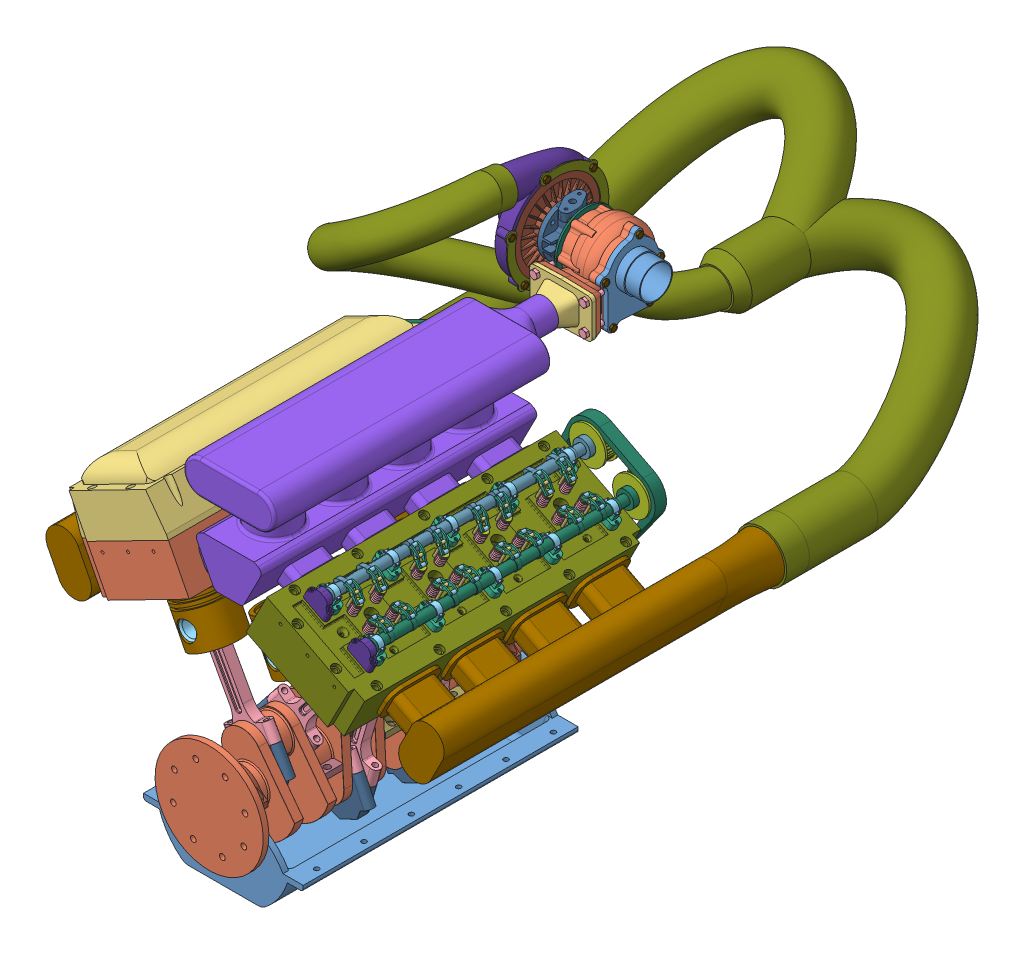
SolidWorks assembly ENSAMBLAJE DE MOTOR V8, configuration Predeterminado. Lengths in mm.
Overall size (718.67 744.91 1254.41).
367 component instances, 54 part files, 489 mates.
Components (placement in the parent):
- BLOQUE V8-1: BLOQUE V8 [Predeterminado] at (-129.263 -163.8973 268.5) size (422.73 344.7 507) (hidden)
- CARTER-1: CARTER [Predeterminado] at (-129.263 -163.8973 268.5) size (280.01 127.77 492.2)
- CIGUEÑAL-1: CIGUEÑAL [Predeterminado] at (-29.5541 -62.6398 687) x (-0.937671 -0.347525 0) z (0 0 1) size (189.6 189.6 554)
- TAPA DE CULATA DERECHO-1: TAPA DE CULATA DERECHO [Predeterminado] at (-262.0137 169.4282 509.5) x (0 0 1) z (-0.890111 -0.455744 0) size (507 100 181.28)
- TAPA DE CULATA IZQUIERDO-1: TAPA DE CULATA IZQUIERDO [Predeterminado] at (233.5589 169.3917 750.5) x (0 0 -1) z (0.890111 -0.455744 0) size (507 100 181.28) (hidden)
- BIELA-4: BIELA [Predeterminado] at (76.4856 71.7664 618.75) x (0.785083 -0.61939 0) z (0 0 1) size (90 198.82 38)
- BULÓN-1: BULÓN [Predeterminado] at (76.4856 71.7664 618.75) x (0.785083 -0.61939 0) z (0 0 1) size (33.8 33.8 75.8)
- COJINETE-1: COJINETE [Predeterminado] at (76.4856 71.7664 618.75) x (0.890111 -0.455744 0) z (0 0 1) size (35.6 35.6 33)
- COJINETE INFERIOR-1: COJINETE INFERIOR [Predeterminado] at (-29.5541 -62.6398 618.75) x (0.890111 -0.455744 0) z (0 0 -1) size (66 33 18)
- COJINETE SUPERIOR-1: COJINETE SUPERIOR [Predeterminado] at (-29.5541 -62.6398 618.75) x (0.890111 -0.455744 0) z (0 0 1) size (66 33 18)
- PISTÓN-1: PISTÓN [Predeterminado] at (62.3575 44.173 618.75) x (0.890111 -0.455744 0) z (0 0 1) size (86 89 88.08)
- SOMBRERETE DE BIELA-1: SOMBRERETE DE BIELA [Predeterminado] at (-29.5541 -62.6398 618.75) x (0.785083 -0.61939 0) z (-0.61939 -0.785083 0) size (90 18.01 61.91)
- BIELA-5: BIELA [Predeterminado] at (75.9097 72.2187 322.75) x (0.787725 -0.616027 0) z (0 0 1) size (90 198.82 38)
- BULÓN-2: BULÓN [Predeterminado] at (75.9097 72.2187 322.75) x (0.787725 -0.616027 0) z (0 0 1) size (33.8 33.8 75.8)
- COJINETE-2: COJINETE [Predeterminado] at (75.9097 72.2187 322.75) x (0.890111 -0.455744 0) z (0 0 1) size (35.6 35.6 33)
- COJINETE INFERIOR-2: COJINETE INFERIOR [Predeterminado] at (-29.5541 -62.6398 322.75) x (0.890111 -0.455744 0) z (0 0 -1) size (66 33 18)
- COJINETE SUPERIOR-2: COJINETE SUPERIOR [Predeterminado] at (-29.5541 -62.6398 322.75) x (0.890111 -0.455744 0) z (0 0 1) size (66 33 18)
- PISTÓN-2: PISTÓN [Predeterminado] at (61.7817 44.6253 322.75) x (0.890111 -0.455744 0) z (0 0 1) size (86 89 88.08)
- SOMBRERETE DE BIELA-2: SOMBRERETE DE BIELA [Predeterminado] at (-29.5541 -62.6398 322.75) x (0.787725 -0.616027 0) z (-0.616027 -0.787725 0) size (90 18.01 61.91)
- BIELA-6: BIELA [Predeterminado] at (-72.3378 9.5283 454.25) x (0.903523 0.428539 0) z (0 0 1) size (90 198.82 38)
- BULÓN-3: BULÓN [Predeterminado] at (-72.3378 9.5283 454.25) x (0.903523 0.428539 0) z (0 0 1) size (33.8 33.8 75.8)
- COJINETE-3: COJINETE [Predeterminado] at (-72.3378 9.5283 454.25) x (0.890111 0.455744 0) z (0 0 1) size (35.6 35.6 33)
- COJINETE INFERIOR-3: COJINETE INFERIOR [Predeterminado] at (1.0281 -145.1549 454.25) x (0.890111 0.455744 0) z (0 0 -1) size (66 33 18)
- COJINETE SUPERIOR-3: COJINETE SUPERIOR [Predeterminado] at (1.0281 -145.1549 454.25) x (0.890111 0.455744 0) z (0 0 1) size (66 33 18)
- PISTÓN-3: PISTÓN [Predeterminado] at (-58.2097 -18.0651 454.25) x (0.890111 0.455744 0) z (0 0 1) size (86 89 88.08)
- SOMBRERETE DE BIELA-3: SOMBRERETE DE BIELA [Predeterminado] at (1.0281 -145.1549 454.25) x (0.903523 0.428539 0) z (0.428539 -0.903523 0) size (90 18.01 61.91)
- BIELA-7: BIELA [Predeterminado] at (71.2823 63.1809 432.75) x (0.970092 -0.242737 0) z (0 0 1) size (90 198.82 38)
- BULÓN-4: BULÓN [Predeterminado] at (71.2823 63.1809 432.75) x (0.970092 -0.242737 0) z (0 0 1) size (33.8 33.8 75.8)
- COJINETE-4: COJINETE [Predeterminado] at (71.2823 63.1809 432.75) x (0.890111 -0.455744 0) z (0 0 1) size (35.6 35.6 33)
- COJINETE INFERIOR-4: COJINETE INFERIOR [Predeterminado] at (29.7257 -102.8988 432.75) x (0.890111 -0.455744 0) z (0 0 -1) size (66 33 18)
- COJINETE SUPERIOR-4: COJINETE SUPERIOR [Predeterminado] at (29.7257 -102.8988 432.75) x (0.890111 -0.455744 0) z (0 0 1) size (66 33 18)
- PISTÓN-4: PISTÓN [Predeterminado] at (57.1543 35.5875 432.75) x (0.890111 -0.455744 0) z (0 0 1) size (86 89 88.08)
- SOMBRERETE DE BIELA-4: SOMBRERETE DE BIELA [Predeterminado] at (29.7257 -102.8988 432.75) x (0.970092 -0.242737 0) z (-0.242737 -0.970092 0) size (90 18.01 61.91)
- BIELA-8: BIELA [Predeterminado] at (-112.163 87.3108 344.25) x (0.87588 0.482529 0) z (0 0 1) size (90 198.82 38)
- BULÓN-5: BULÓN [Predeterminado] at (-112.163 87.3108 344.25) x (0.87588 0.482529 0) z (0 0 1) size (33.8 33.8 75.8)
- COJINETE-5: COJINETE [Predeterminado] at (-112.163 87.3108 344.25) x (0.890111 0.455744 0) z (0 0 1) size (35.6 35.6 33)
- COJINETE INFERIOR-5: COJINETE INFERIOR [Predeterminado] at (-29.5541 -62.6398 344.25) x (0.890111 0.455744 0) z (0 0 -1) size (66 33 18)
- COJINETE SUPERIOR-5: COJINETE SUPERIOR [Predeterminado] at (-29.5541 -62.6398 344.25) x (0.890111 0.455744 0) z (0 0 1) size (66 33 18)
- PISTÓN-5: PISTÓN [Predeterminado] at (-98.035 59.7174 344.25) x (0.890111 0.455744 0) z (0 0 1) size (86 89 88.08)
- SOMBRERETE DE BIELA-5: SOMBRERETE DE BIELA [Predeterminado] at (-29.5541 -62.6398 344.25) x (0.87588 0.482529 0) z (0.482529 -0.87588 0) size (90 18.01 61.91)
- BIELA-9: BIELA [Predeterminado] at (-72.3378 9.5283 564.25) x (0.903523 0.428539 0) z (0 0 1) size (90 198.82 38)
- BULÓN-6: BULÓN [Predeterminado] at (-72.3378 9.5283 564.25) x (0.903523 0.428539 0) z (0 0 1) size (33.8 33.8 75.8)
- COJINETE-6: COJINETE [Predeterminado] at (-72.3378 9.5283 564.25) x (0.890111 0.455744 0) z (0 0 1) size (35.6 35.6 33)
- COJINETE INFERIOR-6: COJINETE INFERIOR [Predeterminado] at (1.0281 -145.1549 564.25) x (0.890111 0.455744 0) z (0 0 -1) size (66 33 18)
- COJINETE SUPERIOR-6: COJINETE SUPERIOR [Predeterminado] at (1.0281 -145.1549 564.25) x (0.890111 0.455744 0) z (0 0 1) size (66 33 18)
- PISTÓN-6: PISTÓN [Predeterminado] at (-58.2097 -18.0651 564.25) x (0.890111 0.455744 0) z (0 0 1) size (86 89 88.08)
- SOMBRERETE DE BIELA-6: SOMBRERETE DE BIELA [Predeterminado] at (1.0281 -145.1549 564.25) x (0.903523 0.428539 0) z (0.428539 -0.903523 0) size (90 18.01 61.91)
- BIELA-10: BIELA [Predeterminado] at (48.7885 19.2483 542.75) x (0.960299 -0.278974 0) z (0 0 1) size (90 198.82 38)
- BULÓN-7: BULÓN [Predeterminado] at (48.7885 19.2483 542.75) x (0.960299 -0.278974 0) z (0 0 1) size (33.8 33.8 75.8)
- COJINETE-7: COJINETE [Predeterminado] at (48.7885 19.2483 542.75) x (0.890111 -0.455744 0) z (0 0 1) size (35.6 35.6 33)
- COJINETE INFERIOR-7: COJINETE INFERIOR [Predeterminado] at (1.0281 -145.1549 542.75) x (0.890111 -0.455744 0) z (0 0 -1) size (66 33 18)
- COJINETE SUPERIOR-7: COJINETE SUPERIOR [Predeterminado] at (1.0281 -145.1549 542.75) x (0.890111 -0.455744 0) z (0 0 1) size (66 33 18)
- PISTÓN-7: PISTÓN [Predeterminado] at (34.6604 -8.3452 542.75) x (0.890111 -0.455744 0) z (0 0 1) size (86 89 88.08)
- SOMBRERETE DE BIELA-7: SOMBRERETE DE BIELA [Predeterminado] at (1.0281 -145.1549 542.75) x (0.960299 -0.278974 0) z (-0.278974 -0.960299 0) size (90 18.01 61.91)
- BIELA-11: BIELA [Predeterminado] at (-112.163 87.3108 676.25) x (0.87588 0.482529 0) z (0 0 1) size (90 198.82 38)
- BULÓN-8: BULÓN [Predeterminado] at (-112.163 87.3108 676.25) x (0.87588 0.482529 0) z (0 0 1) size (33.8 33.8 75.8)
- COJINETE-8: COJINETE [Predeterminado] at (-112.163 87.3108 676.25) x (0.890111 0.455744 0) z (0 0 1) size (35.6 35.6 33)
- COJINETE INFERIOR-8: COJINETE INFERIOR [Predeterminado] at (-29.5541 -62.6398 676.25) x (0.890111 0.455744 0) z (0 0 -1) size (66 33 18)
- COJINETE SUPERIOR-8: COJINETE SUPERIOR [Predeterminado] at (-29.5541 -62.6398 676.25) x (0.890111 0.455744 0) z (0 0 1) size (66 33 18)
- PISTÓN-8: PISTÓN [Predeterminado] at (-98.035 59.7174 676.25) x (0.890111 0.455744 0) z (0 0 1) size (86 89 88.08)
- SOMBRERETE DE BIELA-8: SOMBRERETE DE BIELA [Predeterminado] at (-29.5541 -62.6398 676.25) x (0.87588 0.482529 0) z (0.482529 -0.87588 0) size (90 18.01 61.91)
- SEGURO DE CIGÜEÑAL DE 18mm-1: SEGURO DE CIGÜEÑAL DE 18mm [Predeterminado] at (-14.263 -103.8973 740.5) x (-1 0 0) z (0 0 -1) size (100 42 18)
- SEGURO DE CIGÜEÑAL DE 36mm-1: SEGURO DE CIGÜEÑAL DE 36mm [Predeterminado] at (-14.263 -103.8973 480.5) size (100 42 36)
- SEGURO DE CIGÜEÑAL DE 38mm-1: SEGURO DE CIGÜEÑAL DE 38mm [Predeterminado] at (-14.263 -103.8973 628.5) x (1 0 0) z (0 0 -1) size (100 42 38)
- SEGURO DE CIGÜEÑAL DE 18mm-2: SEGURO DE CIGÜEÑAL DE 18mm [Predeterminado] at (-14.263 -103.8973 296.5) x (-1 0 0) z (0 0 -1) size (100 42 18)
- SEGURO DE CIGÜEÑAL DE 36mm-2: SEGURO DE CIGÜEÑAL DE 36mm [Predeterminado] at (-14.263 -103.8973 406.5) x (1 0 0) z (0 0 -1) size (100 42 36)
- ARBOL DE LEVAS DE ADMISIÓN_IZQUIERDO-2: ARBOL DE LEVAS DE ADMISIÓN_IZQUIERDO [Predeterminado] at (129.8464 248.9794 140.5) x (0 0 -1) z (0.282857 0.959162 0) size (491 30 30)
- ARBOL DE LEVAS DE ESCAPE_IZQUIERDO-2: ARBOL DE LEVAS DE ESCAPE_IZQUIERDO [Predeterminado] at (204.8552 206.8485 140.5) x (0 0 1) z (-0.628385 -0.777902 0) size (491 30 30)
- CULATA_IZQUIERDO-2: CULATA_IZQUIERDO [Predeterminado] at (178.4783 107.717 760.5) x (0 0 -1) z (0.890111 -0.455744 0) size (507 80 181.28)
- SOPORTE EXTERNO DE ARBOL DE LEVAS-1: SOPORTE EXTERNO DE ARBOL DE LEVAS [Predeterminado] at (111.6671 231.8013 707.5) x (0.890111 -0.455744 0) z (0 0 1) size (45 34 11)
- SOPORTE EXTERNO DE ARBOL DE LEVAS-2: SOPORTE EXTERNO DE ARBOL DE LEVAS [Predeterminado] at (188.2167 192.6073 707.5) x (0.890111 -0.455744 0) z (0 0 1) size (45 34 11)
- ARBOL DE LEVAS DE ADMISIÓN_DERECHO-1: ARBOL DE LEVAS DE ADMISIÓN_DERECHO [Predeterminado] at (-142.5063 255.1417 153.25) x (0 0 1) z (0.43783 -0.899058 0) size (511.75 30 30)
- ARBOL DE LEVAS DE ESCAPE_DERECHO-1: ARBOL DE LEVAS DE ESCAPE_DERECHO [Predeterminado] at (-218.2013 211.9839 153.25) x (0 0 -1) z (0.028509 0.999594 0) size (511.75 30 30)
- CULATA_DERECHO-1: CULATA_DERECHO [Predeterminado] at (-64.1949 180.8365 253.5) x (0 0 1) z (-0.890111 -0.455744 0) size (507 80 181.28)
- SOPORTE EXTERNO DE ARBOL DE LEVAS-3: SOPORTE EXTERNO DE ARBOL DE LEVAS [Predeterminado] at (-216.6715 192.6438 728.25) x (0.890111 0.455744 0) z (0 0 1) size (45 34 11)
- SOPORTE EXTERNO DE ARBOL DE LEVAS-4: SOPORTE EXTERNO DE ARBOL DE LEVAS [Predeterminado] at (-140.1219 231.8377 728.25) x (0.890111 0.455744 0) z (0 0 1) size (45 34 11)
- EJE DE CONTROL DE VÁLVULAS-1: EJE DE CONTROL DE VÁLVULAS [Predeterminado] at (-159.7346 199.2777 696.25) x (0 0 -1) z (0.890111 0.455744 0) size (14 48.5 5)
- RESORTE DE VÁLVULA-1: RESORTE DE VÁLVULA [Predeterminado] at (-160.667 210.5262 696.25) x (0 0 -1) z (0.890111 0.455744 0) size (15.13 32.27 14.6)
- SEGUIDOR DE LEVA-1: SEGUIDOR DE LEVA [Predeterminado] at (-166.3151 243.7387 692.45) x (0.994346 0.106192 0) z (0 0 1) size (6 6 7.6)
- SOPORTE DE SEGUIDOR DE VÁLVULA-1: SOPORTE DE SEGUIDOR DE VÁLVULA [Predeterminado] at (-180.6988 240.2228 689.45) x (0.999362 0.035708 0) z (0 0 1) size (30.5 14.83 13.6)
- VÁLVULA-1: VÁLVULA [Predeterminado] at (-129.448 149.5524 696.25) x (0.279369 0.143039 -0.94947) z (0.845134 0.432715 0.313858) size (28 102 28)
- SEGUIDOR DE LEVA-13: SEGUIDOR DE LEVA [Predeterminado] at (-191.9772 233.816 692.45) x (1 0 0) z (0 0 1) size (6 6 7.6)
- EJE DE CONTROL DE VÁLVULAS-2: EJE DE CONTROL DE VÁLVULAS [Predeterminado] at (-149.3077 210.2827 584.25) x (0 0 -1) z (0.890111 0.455744 0) size (14 48.5 5)
- RESORTE DE VÁLVULA-2: RESORTE DE VÁLVULA [Predeterminado] at (-160.3993 210.0033 584.25) x (0 0 -1) z (0.890111 0.455744 0) size (15.13 32.27 14.6)
- SEGUIDOR DE LEVA-17: SEGUIDOR DE LEVA [Predeterminado] at (-158.8913 260.7004 580.45) x (-0.483729 0.875218 0) z (0 0 1) size (6 6 7.6)
- SOPORTE DE SEGUIDOR DE VÁLVULA-2: SOPORTE DE SEGUIDOR DE VÁLVULA [Predeterminado] at (-170.2719 251.2278 577.45) x (0.88227 0.470744 0) z (0 0 1) size (30.5 14.83 13.6)
- VÁLVULA-2: VÁLVULA [Predeterminado] at (-129.1802 149.0296 584.25) x (0.372659 0.190804 -0.908141) z (0.808346 0.413879 0.418665) size (28 102 28)
- SEGUIDOR DE LEVA-21: SEGUIDOR DE LEVA [Predeterminado] at (-177.5936 240.5206 580.45) size (6 6 7.6)
- SEGUIDOR DE LEVA-5: SEGUIDOR DE LEVA [Predeterminado] at (-166.3151 243.7387 652.45) x (0.994346 0.106192 0) z (0 0 1) size (6 6 7.6)
- EJE DE CONTROL DE VÁLVULAS-3: EJE DE CONTROL DE VÁLVULAS [Predeterminado] at (-159.7346 199.2777 656.25) x (0 0 -1) z (0.890111 0.455744 0) size (14 48.5 5)
- SOPORTE DE SEGUIDOR DE VÁLVULA-3: SOPORTE DE SEGUIDOR DE VÁLVULA [Predeterminado] at (-180.6988 240.2228 649.45) x (0.999362 0.035708 0) z (0 0 1) size (30.5 14.83 13.6)
- RESORTE DE VÁLVULA-3: RESORTE DE VÁLVULA [Predeterminado] at (-160.667 210.5262 656.25) x (0 0 -1) z (0.890111 0.455744 0) size (15.13 32.27 14.6)
- VÁLVULA-3: VÁLVULA [Predeterminado] at (-129.448 149.5524 656.25) x (0.279369 0.143039 -0.94947) z (0.845134 0.432715 0.313858) size (28 102 28)
- SEGUIDOR DE LEVA-14: SEGUIDOR DE LEVA [Predeterminado] at (-191.9772 233.816 652.45) x (1 0 0) z (0 0 1) size (6 6 7.6)
- SEGUIDOR DE LEVA-18: SEGUIDOR DE LEVA [Predeterminado] at (-158.8913 260.7004 540.45) x (-0.483729 0.875218 0) z (0 0 1) size (6 6 7.6)
- EJE DE CONTROL DE VÁLVULAS-4: EJE DE CONTROL DE VÁLVULAS [Predeterminado] at (-149.3077 210.2827 544.25) x (0 0 -1) z (0.890111 0.455744 0) size (14 48.5 5)
- SOPORTE DE SEGUIDOR DE VÁLVULA-4: SOPORTE DE SEGUIDOR DE VÁLVULA [Predeterminado] at (-170.2719 251.2278 537.45) x (0.88227 0.470744 0) z (0 0 1) size (30.5 14.83 13.6)
- VÁLVULA-4: VÁLVULA [Predeterminado] at (-129.1802 149.0296 544.25) x (0.372659 0.190804 -0.908141) z (0.808346 0.413879 0.418665) size (28 102 28)
- SEGUIDOR DE LEVA-22: SEGUIDOR DE LEVA [Predeterminado] at (-177.5936 240.5206 540.45) size (6 6 7.6)
- RESORTE DE VÁLVULA-4: RESORTE DE VÁLVULA [Predeterminado] at (-160.3993 210.0033 544.25) x (0 0 -1) z (0.890111 0.455744 0) size (15.13 32.27 14.6)
- SEGUIDOR DE LEVA-12: SEGUIDOR DE LEVA [Predeterminado] at (-166.3151 243.7387 360.45) x (0.994346 0.106192 0) z (0 0 1) size (6 6 7.6)
- EJE DE CONTROL DE VÁLVULAS-5: EJE DE CONTROL DE VÁLVULAS [Predeterminado] at (-159.7346 199.2777 364.25) x (0 0 -1) z (0.890111 0.455744 0) size (14 48.5 5)
- SOPORTE DE SEGUIDOR DE VÁLVULA-5: SOPORTE DE SEGUIDOR DE VÁLVULA [Predeterminado] at (-180.6988 240.2228 357.45) x (0.999362 0.035708 0) z (0 0 1) size (30.5 14.83 13.6)
- RESORTE DE VÁLVULA-5: RESORTE DE VÁLVULA [Predeterminado] at (-160.667 210.5262 364.25) x (0 0 -1) z (0.890111 0.455744 0) size (15.13 32.27 14.6)
- VÁLVULA-5: VÁLVULA [Predeterminado] at (-129.448 149.5524 364.25) x (0.279369 0.143039 -0.94947) z (0.845134 0.432715 0.313858) size (28 102 28)
- SEGUIDOR DE LEVA-16: SEGUIDOR DE LEVA [Predeterminado] at (-191.9772 233.816 360.45) x (1 0 0) z (0 0 1) size (6 6 7.6)
- SEGUIDOR DE LEVA-11: SEGUIDOR DE LEVA [Predeterminado] at (-166.3151 243.7387 320.45) x (0.994346 0.106192 0) z (0 0 1) size (6 6 7.6)
- EJE DE CONTROL DE VÁLVULAS-6: EJE DE CONTROL DE VÁLVULAS [Predeterminado] at (-159.7346 199.2777 324.25) x (0 0 -1) z (0.890111 0.455744 0) size (14 48.5 5)
- SOPORTE DE SEGUIDOR DE VÁLVULA-6: SOPORTE DE SEGUIDOR DE VÁLVULA [Predeterminado] at (-180.6988 240.2228 317.45) x (0.999362 0.035708 0) z (0 0 1) size (30.5 14.83 13.6)
- RESORTE DE VÁLVULA-6: RESORTE DE VÁLVULA [Predeterminado] at (-160.667 210.5262 324.25) x (0 0 -1) z (0.890111 0.455744 0) size (15.13 32.27 14.6)
- VÁLVULA-6: VÁLVULA [Predeterminado] at (-129.448 149.5524 324.25) x (0.279369 0.143039 -0.94947) z (0.845134 0.432715 0.313858) size (28 102 28)
- SEGUIDOR DE LEVA-15: SEGUIDOR DE LEVA [Predeterminado] at (-191.9772 233.816 320.45) x (1 0 0) z (0 0 1) size (6 6 7.6)
- SEGUIDOR DE LEVA-20: SEGUIDOR DE LEVA [Predeterminado] at (-158.8913 260.7004 470.45) x (-0.483729 0.875218 0) z (0 0 1) size (6 6 7.6)
- EJE DE CONTROL DE VÁLVULAS-7: EJE DE CONTROL DE VÁLVULAS [Predeterminado] at (-149.3077 210.2827 474.25) x (0 0 -1) z (0.890111 0.455744 0) size (14 48.5 5)
- SOPORTE DE SEGUIDOR DE VÁLVULA-7: SOPORTE DE SEGUIDOR DE VÁLVULA [Predeterminado] at (-170.2719 251.2278 467.45) x (0.88227 0.470744 0) z (0 0 1) size (30.5 14.83 13.6)
- VÁLVULA-7: VÁLVULA [Predeterminado] at (-129.1802 149.0296 474.25) x (0.372659 0.190804 -0.908141) z (0.808346 0.413879 0.418665) size (28 102 28)
- SEGUIDOR DE LEVA-24: SEGUIDOR DE LEVA [Predeterminado] at (-177.5936 240.5206 470.45) size (6 6 7.6)
- RESORTE DE VÁLVULA-7: RESORTE DE VÁLVULA [Predeterminado] at (-160.3993 210.0033 474.25) x (0 0 -1) z (0.890111 0.455744 0) size (15.13 32.27 14.6)
- SEGUIDOR DE LEVA-19: SEGUIDOR DE LEVA [Predeterminado] at (-158.8913 260.7004 430.45) x (-0.483729 0.875218 0) z (0 0 1) size (6 6 7.6)
- EJE DE CONTROL DE VÁLVULAS-8: EJE DE CONTROL DE VÁLVULAS [Predeterminado] at (-149.3077 210.2827 434.25) x (0 0 -1) z (0.890111 0.455744 0) size (14 48.5 5)
- SOPORTE DE SEGUIDOR DE VÁLVULA-8: SOPORTE DE SEGUIDOR DE VÁLVULA [Predeterminado] at (-170.2719 251.2278 427.45) x (0.88227 0.470744 0) z (0 0 1) size (30.5 14.83 13.6)
- VÁLVULA-8: VÁLVULA [Predeterminado] at (-129.1802 149.0296 434.25) x (0.372659 0.190804 -0.908141) z (0.808346 0.413879 0.418665) size (28 102 28)
- SEGUIDOR DE LEVA-23: SEGUIDOR DE LEVA [Predeterminado] at (-177.5936 240.5206 430.45) size (6 6 7.6)
- RESORTE DE VÁLVULA-8: RESORTE DE VÁLVULA [Predeterminado] at (-160.3993 210.0033 434.25) x (0 0 -1) z (0.890111 0.455744 0) size (15.13 32.27 14.6)
- EJE DE CONTROL DE VÁLVULAS-9: EJE DE CONTROL DE VÁLVULAS [Predeterminado] at (-193.8133 187.4955 696.25) x (0 0 1) z (-0.890111 -0.455744 0) size (14 48.5 5)
- RESORTE DE VÁLVULA-9: RESORTE DE VÁLVULA [Predeterminado] at (-187.3703 196.8538 696.25) x (0.890111 0.455744 0) z (0 0 1) size (15.13 32.27 14.6)
- SEGUIDOR DE LEVA-25: SEGUIDOR DE LEVA [Predeterminado] at (-201.8109 228.7811 700.05) x (0.255826 0.966723 0) z (0 0 -1) size (6 6 7.6)
- SOPORTE DE SEGUIDOR DE VÁLVULA-9: SOPORTE DE SEGUIDOR DE VÁLVULA [Predeterminado] at (-214.7775 228.4406 703.05) x (-0.874136 -0.485681 0) z (0 0 -1) size (30.5 14.83 13.6)
- VÁLVULA-9: VÁLVULA [Predeterminado] at (-156.1513 135.8801 696.25) x (-0.890004 -0.455689 0.015535) z (-0.013828 -0.00708 -0.999879) size (28 102 28)
- SEGUIDOR DE LEVA-34: SEGUIDOR DE LEVA [Predeterminado] at (-228.9095 224.0206 700.05) x (0.999498 -0.031694 0) z (0 0 -1) size (6 6 7.6)
- EJE DE CONTROL DE VÁLVULAS-10: EJE DE CONTROL DE VÁLVULAS [Predeterminado] at (-193.8133 187.4955 584.25) x (0 0 -1) z (0.890111 0.455744 0) size (14 48.5 5)
- RESORTE DE VÁLVULA-10: RESORTE DE VÁLVULA [Predeterminado] at (-187.8751 197.8398 584.25) x (0.873481 0.447229 0.192399) z (-0.171257 -0.087685 0.981317) size (15.13 32.27 14.6)
- SEGUIDOR DE LEVA-38: SEGUIDOR DE LEVA [Predeterminado] at (-228.4393 222.7305 588.05) x (-0.584591 -0.811328 0) z (0 0 -1) size (6 6 7.6)
- SOPORTE DE SEGUIDOR DE VÁLVULA-10: SOPORTE DE SEGUIDOR DE VÁLVULA [Predeterminado] at (-214.7775 228.4406 591.05) x (-0.825387 -0.564567 0) z (0 0 -1) size (30.5 14.83 13.6)
- VÁLVULA-10: VÁLVULA [Predeterminado] at (-156.6561 136.866 584.25) x (0.890111 0.455744 0) z (0 0 1) size (28 102 28)
- SEGUIDOR DE LEVA-42: SEGUIDOR DE LEVA [Predeterminado] at (-201.8981 229.9808 580.45) size (6 6 7.6)
- RESORTE DE VÁLVULA-11: RESORTE DE VÁLVULA [Predeterminado] at (-187.3703 196.8538 656.25) x (0.890111 0.455744 0) z (0 0 1) size (15.13 32.27 14.6) (hidden)
- VÁLVULA-11: VÁLVULA [Predeterminado] at (-156.1513 135.8801 656.25) x (-0.890004 -0.455689 0.015535) z (-0.013828 -0.00708 -0.999879) size (28 102 28) (hidden)
- SEGUIDOR DE LEVA-35: SEGUIDOR DE LEVA [Predeterminado] at (-228.9095 224.0206 660.05) x (0.999498 -0.031694 0) z (0 0 -1) size (6 6 7.6)
- SEGUIDOR DE LEVA-26: SEGUIDOR DE LEVA [Predeterminado] at (-201.8109 228.7811 660.05) x (0.255826 0.966723 0) z (0 0 -1) size (6 6 7.6)
- SOPORTE DE SEGUIDOR DE VÁLVULA-11: SOPORTE DE SEGUIDOR DE VÁLVULA [Predeterminado] at (-214.7775 228.4406 663.05) x (-0.874136 -0.485681 0) z (0 0 -1) size (30.5 14.83 13.6)
- EJE DE CONTROL DE VÁLVULAS-11: EJE DE CONTROL DE VÁLVULAS [Predeterminado] at (-193.8133 187.4955 656.25) x (0 0 1) z (-0.890111 -0.455744 0) size (14 48.5 5)
- VÁLVULA-12: VÁLVULA [Predeterminado] at (-156.6561 136.866 544.25) x (0.890111 0.455744 0) z (0 0 1) size (28 102 28)
- RESORTE DE VÁLVULA-12: RESORTE DE VÁLVULA [Predeterminado] at (-187.8751 197.8398 544.25) x (0.873481 0.447229 0.192399) z (-0.171257 -0.087685 0.981317) size (15.13 32.27 14.6)
- SOPORTE DE SEGUIDOR DE VÁLVULA-12: SOPORTE DE SEGUIDOR DE VÁLVULA [Predeterminado] at (-214.7775 228.4406 551.05) x (-0.825387 -0.564567 0) z (0 0 -1) size (30.5 14.83 13.6)
- SEGUIDOR DE LEVA-39: SEGUIDOR DE LEVA [Predeterminado] at (-228.4393 222.7305 548.05) x (-0.584591 -0.811328 0) z (0 0 -1) size (6 6 7.6)
- EJE DE CONTROL DE VÁLVULAS-12: EJE DE CONTROL DE VÁLVULAS [Predeterminado] at (-193.8133 187.4955 544.25) x (0 0 -1) z (0.890111 0.455744 0) size (14 48.5 5)
- SEGUIDOR DE LEVA-43: SEGUIDOR DE LEVA [Predeterminado] at (-201.8981 229.9808 540.45) size (6 6 7.6)
- VÁLVULA-13: VÁLVULA [Predeterminado] at (-156.6561 136.866 474.25) x (0.890111 0.455744 0) z (0 0 1) size (28 102 28)
- RESORTE DE VÁLVULA-13: RESORTE DE VÁLVULA [Predeterminado] at (-187.8751 197.8398 474.25) x (0.873481 0.447229 0.192399) z (-0.171257 -0.087685 0.981317) size (15.13 32.27 14.6)
- SOPORTE DE SEGUIDOR DE VÁLVULA-13: SOPORTE DE SEGUIDOR DE VÁLVULA [Predeterminado] at (-214.7775 228.4406 481.05) x (-0.825387 -0.564567 0) z (0 0 -1) size (30.5 14.83 13.6)
- SEGUIDOR DE LEVA-41: SEGUIDOR DE LEVA [Predeterminado] at (-228.4393 222.7305 478.05) x (-0.584591 -0.811328 0) z (0 0 -1) size (6 6 7.6)
- EJE DE CONTROL DE VÁLVULAS-13: EJE DE CONTROL DE VÁLVULAS [Predeterminado] at (-193.8133 187.4955 474.25) x (0 0 -1) z (0.890111 0.455744 0) size (14 48.5 5)
- SEGUIDOR DE LEVA-45: SEGUIDOR DE LEVA [Predeterminado] at (-201.8981 229.9808 470.45) size (6 6 7.6)
- VÁLVULA-14: VÁLVULA [Predeterminado] at (-156.6561 136.866 434.25) x (0.890111 0.455744 0) z (0 0 1) size (28 102 28)
- RESORTE DE VÁLVULA-14: RESORTE DE VÁLVULA [Predeterminado] at (-187.8751 197.8398 434.25) x (0.873481 0.447229 0.192399) z (-0.171257 -0.087685 0.981317) size (15.13 32.27 14.6)
- SOPORTE DE SEGUIDOR DE VÁLVULA-14: SOPORTE DE SEGUIDOR DE VÁLVULA [Predeterminado] at (-214.7775 228.4406 441.05) x (-0.825387 -0.564567 0) z (0 0 -1) size (30.5 14.83 13.6)
- SEGUIDOR DE LEVA-40: SEGUIDOR DE LEVA [Predeterminado] at (-228.4393 222.7305 438.05) x (-0.584591 -0.811328 0) z (0 0 -1) size (6 6 7.6)
- EJE DE CONTROL DE VÁLVULAS-14: EJE DE CONTROL DE VÁLVULAS [Predeterminado] at (-193.8133 187.4955 434.25) x (0 0 -1) z (0.890111 0.455744 0) size (14 48.5 5)
- SEGUIDOR DE LEVA-44: SEGUIDOR DE LEVA [Predeterminado] at (-201.8981 229.9808 430.45) size (6 6 7.6)
- RESORTE DE VÁLVULA-15: RESORTE DE VÁLVULA [Predeterminado] at (-187.3703 196.8538 364.25) x (0.890111 0.455744 0) z (0 0 1) size (15.13 32.27 14.6)
- VÁLVULA-15: VÁLVULA [Predeterminado] at (-156.1513 135.8801 364.25) x (-0.890004 -0.455689 0.015535) z (-0.013828 -0.00708 -0.999879) size (28 102 28)
- SEGUIDOR DE LEVA-37: SEGUIDOR DE LEVA [Predeterminado] at (-228.9095 224.0206 368.05) x (0.999498 -0.031694 0) z (0 0 -1) size (6 6 7.6)
- SEGUIDOR DE LEVA-33: SEGUIDOR DE LEVA [Predeterminado] at (-201.8109 228.7811 368.05) x (0.255826 0.966723 0) z (0 0 -1) size (6 6 7.6)
- SOPORTE DE SEGUIDOR DE VÁLVULA-15: SOPORTE DE SEGUIDOR DE VÁLVULA [Predeterminado] at (-214.7775 228.4406 371.05) x (-0.874136 -0.485681 0) z (0 0 -1) size (30.5 14.83 13.6)
- EJE DE CONTROL DE VÁLVULAS-15: EJE DE CONTROL DE VÁLVULAS [Predeterminado] at (-193.8133 187.4955 364.25) x (0 0 1) z (-0.890111 -0.455744 0) size (14 48.5 5)
- RESORTE DE VÁLVULA-16: RESORTE DE VÁLVULA [Predeterminado] at (-187.3703 196.8538 324.25) x (0.890111 0.455744 0) z (0 0 1) size (15.13 32.27 14.6)
- VÁLVULA-16: VÁLVULA [Predeterminado] at (-156.1513 135.8801 324.25) x (-0.890004 -0.455689 0.015535) z (-0.013828 -0.00708 -0.999879) size (28 102 28)
- SEGUIDOR DE LEVA-36: SEGUIDOR DE LEVA [Predeterminado] at (-228.9095 224.0206 328.05) x (0.999498 -0.031694 0) z (0 0 -1) size (6 6 7.6)
- SEGUIDOR DE LEVA-32: SEGUIDOR DE LEVA [Predeterminado] at (-201.8109 228.7811 328.05) x (0.255826 0.966723 0) z (0 0 -1) size (6 6 7.6)
- SOPORTE DE SEGUIDOR DE VÁLVULA-16: SOPORTE DE SEGUIDOR DE VÁLVULA [Predeterminado] at (-214.7775 228.4406 331.05) x (-0.874136 -0.485681 0) z (0 0 -1) size (30.5 14.83 13.6)
- EJE DE CONTROL DE VÁLVULAS-16: EJE DE CONTROL DE VÁLVULAS [Predeterminado] at (-193.8133 187.4955 324.25) x (0 0 1) z (-0.890111 -0.455744 0) size (14 48.5 5)
- EJE DE CONTROL DE VÁLVULAS-17: EJE DE CONTROL DE VÁLVULAS [Predeterminado] at (165.3585 187.459 302.75) x (0 0 -1) z (0.890111 -0.455744 0) size (14 48.5 5)
- RESORTE DE VÁLVULA-17: RESORTE DE VÁLVULA [Predeterminado] at (158.8578 196.7046 302.75) x (0.890111 -0.455744 0) z (0 0 1) size (15.13 32.27 14.6)
- VÁLVULA-18: VÁLVULA [Predeterminado] at (127.6388 135.7308 302.75) x (-0.366338 0.187568 0.911381) z (-0.81123 0.415356 -0.411564) size (28 102 28)
- SEGUIDOR DE LEVA-46: SEGUIDOR DE LEVA [Predeterminado] at (200.5019 224.138 298.95) x (0.783614 -0.621248 0) z (0 0 1) size (6 6 7.6)
- SOPORTE DE SEGUIDOR DE VÁLVULA-19: SOPORTE DE SEGUIDOR DE VÁLVULA [Predeterminado] at (186.3227 228.4041 295.95) x (0.879361 -0.476156 0) z (0 0 1) size (30.5 14.83 13.6)
- SEGUIDOR DE LEVA-53: SEGUIDOR DE LEVA [Predeterminado] at (173.3532 228.6038 298.95) size (6 6 7.6)
- EJE DE CONTROL DE VÁLVULAS-19: EJE DE CONTROL DE VÁLVULAS [Predeterminado] at (165.3585 187.459 412.75) x (0 0 1) z (-0.890111 0.455744 0) size (14 48.5 5)
- RESORTE DE VÁLVULA-19: RESORTE DE VÁLVULA [Predeterminado] at (158.6478 196.2945 412.75) x (0 0 1) z (-0.890111 0.455744 0) size (15.13 32.27 14.6)
- SEGUIDOR DE LEVA-57: SEGUIDOR DE LEVA [Predeterminado] at (200.6612 224.7083 408.95) size (6 6 7.6)
- SOPORTE DE SEGUIDOR DE VÁLVULA-21: SOPORTE DE SEGUIDOR DE VÁLVULA [Predeterminado] at (186.3227 228.4041 405.95) x (0.897697 -0.440613 0) z (0 0 1) size (30.5 14.83 13.6)
- VÁLVULA-20: VÁLVULA [Predeterminado] at (127.4288 135.3208 412.75) x (0.832766 -0.426382 0.353127) z (-0.314323 0.160936 0.935575) size (28 102 28)
- SEGUIDOR DE LEVA-61: SEGUIDOR DE LEVA [Predeterminado] at (173.3555 228.085 408.95) size (6 6 7.6)
- RESORTE DE VÁLVULA-20: RESORTE DE VÁLVULA [Predeterminado] at (158.8578 196.7046 342.75) x (0.890111 -0.455744 0) z (0 0 1) size (15.13 32.27 14.6)
- VÁLVULA-21: VÁLVULA [Predeterminado] at (127.6388 135.7308 342.75) x (-0.366338 0.187568 0.911381) z (-0.81123 0.415356 -0.411564) size (28 102 28)
- SOPORTE DE SEGUIDOR DE VÁLVULA-22: SOPORTE DE SEGUIDOR DE VÁLVULA [Predeterminado] at (186.3227 228.4041 335.95) x (0.879361 -0.476156 0) z (0 0 1) size (30.5 14.83 13.6)
- SEGUIDOR DE LEVA-54: SEGUIDOR DE LEVA [Predeterminado] at (173.3532 228.6038 338.95) size (6 6 7.6)
- EJE DE CONTROL DE VÁLVULAS-20: EJE DE CONTROL DE VÁLVULAS [Predeterminado] at (165.3585 187.459 342.75) x (0 0 -1) z (0.890111 -0.455744 0) size (14 48.5 5)
- SEGUIDOR DE LEVA-47: SEGUIDOR DE LEVA [Predeterminado] at (200.5019 224.138 338.95) x (0.783614 -0.621248 0) z (0 0 1) size (6 6 7.6)
- RESORTE DE VÁLVULA-21: RESORTE DE VÁLVULA [Predeterminado] at (158.6478 196.2945 452.75) x (0 0 1) z (-0.890111 0.455744 0) size (15.13 32.27 14.6)
- VÁLVULA-22: VÁLVULA [Predeterminado] at (127.4288 135.3208 452.75) x (0.832766 -0.426382 0.353127) z (-0.314323 0.160936 0.935575) size (28 102 28)
- SEGUIDOR DE LEVA-62: SEGUIDOR DE LEVA [Predeterminado] at (173.3555 228.085 448.95) size (6 6 7.6)
- SEGUIDOR DE LEVA-58: SEGUIDOR DE LEVA [Predeterminado] at (200.6612 224.7083 448.95) size (6 6 7.6)
- SOPORTE DE SEGUIDOR DE VÁLVULA-23: SOPORTE DE SEGUIDOR DE VÁLVULA [Predeterminado] at (186.3227 228.4041 445.95) x (0.897697 -0.440613 0) z (0 0 1) size (30.5 14.83 13.6)
- EJE DE CONTROL DE VÁLVULAS-21: EJE DE CONTROL DE VÁLVULAS [Predeterminado] at (165.3585 187.459 452.75) x (0 0 1) z (-0.890111 0.455744 0) size (14 48.5 5)
- RESORTE DE VÁLVULA-22: RESORTE DE VÁLVULA [Predeterminado] at (158.6478 196.2945 522.75) x (0 0 1) z (-0.890111 0.455744 0) size (15.13 32.27 14.6)
- VÁLVULA-23: VÁLVULA [Predeterminado] at (127.4288 135.3208 522.75) x (0.832766 -0.426382 0.353127) z (-0.314323 0.160936 0.935575) size (28 102 28)
- SEGUIDOR DE LEVA-64: SEGUIDOR DE LEVA [Predeterminado] at (173.3555 228.085 518.95) size (6 6 7.6)
- SEGUIDOR DE LEVA-60: SEGUIDOR DE LEVA [Predeterminado] at (200.6612 224.7083 518.95) size (6 6 7.6)
- SOPORTE DE SEGUIDOR DE VÁLVULA-24: SOPORTE DE SEGUIDOR DE VÁLVULA [Predeterminado] at (186.3227 228.4041 515.95) x (0.897697 -0.440613 0) z (0 0 1) size (30.5 14.83 13.6)
- EJE DE CONTROL DE VÁLVULAS-22: EJE DE CONTROL DE VÁLVULAS [Predeterminado] at (165.3585 187.459 522.75) x (0 0 1) z (-0.890111 0.455744 0) size (14 48.5 5)
- RESORTE DE VÁLVULA-23: RESORTE DE VÁLVULA [Predeterminado] at (158.6478 196.2945 562.75) x (0 0 1) z (-0.890111 0.455744 0) size (15.13 32.27 14.6)
- VÁLVULA-24: VÁLVULA [Predeterminado] at (127.4288 135.3208 562.75) x (0.832766 -0.426382 0.353127) z (-0.314323 0.160936 0.935575) size (28 102 28)
- SEGUIDOR DE LEVA-63: SEGUIDOR DE LEVA [Predeterminado] at (173.3555 228.085 558.95) size (6 6 7.6)
- SEGUIDOR DE LEVA-59: SEGUIDOR DE LEVA [Predeterminado] at (200.6612 224.7083 558.95) size (6 6 7.6)
- SOPORTE DE SEGUIDOR DE VÁLVULA-25: SOPORTE DE SEGUIDOR DE VÁLVULA [Predeterminado] at (186.3227 228.4041 555.95) x (0.897697 -0.440613 0) z (0 0 1) size (30.5 14.83 13.6)
- EJE DE CONTROL DE VÁLVULAS-23: EJE DE CONTROL DE VÁLVULAS [Predeterminado] at (165.3585 187.459 562.75) x (0 0 1) z (-0.890111 0.455744 0) size (14 48.5 5)
- RESORTE DE VÁLVULA-24: RESORTE DE VÁLVULA [Predeterminado] at (158.8578 196.7046 634.75) x (0.890111 -0.455744 0) z (0 0 1) size (15.13 32.27 14.6)
- VÁLVULA-25: VÁLVULA [Predeterminado] at (127.6388 135.7308 634.75) x (-0.366338 0.187568 0.911381) z (-0.81123 0.415356 -0.411564) size (28 102 28)
- SOPORTE DE SEGUIDOR DE VÁLVULA-26: SOPORTE DE SEGUIDOR DE VÁLVULA [Predeterminado] at (186.3227 228.4041 627.95) x (0.879361 -0.476156 0) z (0 0 1) size (30.5 14.83 13.6)
- SEGUIDOR DE LEVA-56: SEGUIDOR DE LEVA [Predeterminado] at (173.3532 228.6038 630.95) size (6 6 7.6)
- EJE DE CONTROL DE VÁLVULAS-24: EJE DE CONTROL DE VÁLVULAS [Predeterminado] at (165.3585 187.459 634.75) x (0 0 -1) z (0.890111 -0.455744 0) size (14 48.5 5)
- SEGUIDOR DE LEVA-52: SEGUIDOR DE LEVA [Predeterminado] at (200.5019 224.138 630.95) x (0.783614 -0.621248 0) z (0 0 1) size (6 6 7.6)
- RESORTE DE VÁLVULA-25: RESORTE DE VÁLVULA [Predeterminado] at (158.8578 196.7046 674.75) x (0.890111 -0.455744 0) z (0 0 1) size (15.13 32.27 14.6)
- VÁLVULA-26: VÁLVULA [Predeterminado] at (127.6388 135.7308 674.75) x (-0.366338 0.187568 0.911381) z (-0.81123 0.415356 -0.411564) size (28 102 28)
- SOPORTE DE SEGUIDOR DE VÁLVULA-27: SOPORTE DE SEGUIDOR DE VÁLVULA [Predeterminado] at (186.3227 228.4041 667.95) x (0.879361 -0.476156 0) z (0 0 1) size (30.5 14.83 13.6)
- SEGUIDOR DE LEVA-55: SEGUIDOR DE LEVA [Predeterminado] at (173.3532 228.6038 670.95) size (6 6 7.6)
- EJE DE CONTROL DE VÁLVULAS-25: EJE DE CONTROL DE VÁLVULAS [Predeterminado] at (165.3585 187.459 674.75) x (0 0 -1) z (0.890111 -0.455744 0) size (14 48.5 5)
- SEGUIDOR DE LEVA-51: SEGUIDOR DE LEVA [Predeterminado] at (200.5019 224.138 670.95) x (0.783614 -0.621248 0) z (0 0 1) size (6 6 7.6)
- EJE DE CONTROL DE VÁLVULAS-26: EJE DE CONTROL DE VÁLVULAS [Predeterminado] at (120.853 210.2462 674.75) x (0 0 -1) z (0.890111 -0.455744 0) size (14 48.5 5)
- RESORTE DE VÁLVULA-26: RESORTE DE VÁLVULA [Predeterminado] at (132.2122 210.4897 674.75) x (0.361373 -0.185026 -0.913879) z (0.813454 -0.416495 0.405986) size (15.13 32.27 14.6)
- SEGUIDOR DE LEVA-65: SEGUIDOR DE LEVA [Predeterminado] at (129.9696 260.0731 678.55) x (-0.584596 0.811325 0) z (0 0 -1) size (6 6 7.6)
- SOPORTE DE SEGUIDOR DE VÁLVULA-28: SOPORTE DE SEGUIDOR DE VÁLVULA [Predeterminado] at (141.8172 251.1913 681.55) x (-0.905061 0.425281 0) z (0 0 -1) size (30.5 14.83 13.6)
- VÁLVULA-27: VÁLVULA [Predeterminado] at (100.9932 149.516 674.75) x (0.601254 -0.307846 -0.737377) z (0.656347 -0.336055 0.675482) size (28 102 28)
- SEGUIDOR DE LEVA-69: SEGUIDOR DE LEVA [Predeterminado] at (149.6737 240.8702 670.95) size (6 6 7.6)
- EJE DE CONTROL DE VÁLVULAS-27: EJE DE CONTROL DE VÁLVULAS [Predeterminado] at (120.853 210.2462 562.75) x (0 0 -1) z (0.890111 -0.455744 0) size (14 48.5 5)
- RESORTE DE VÁLVULA-27: RESORTE DE VÁLVULA [Predeterminado] at (131.0476 208.2152 562.75) x (0.851719 -0.436086 -0.290524) z (0.258599 -0.132404 0.956868) size (15.13 32.27 14.6)
- SEGUIDOR DE LEVA-73: SEGUIDOR DE LEVA [Predeterminado] at (147.0712 239.3319 566.55) x (0.536876 -0.843661 0) z (0 0 -1) size (6 6 7.6)
- SOPORTE DE SEGUIDOR DE VÁLVULA-29: SOPORTE DE SEGUIDOR DE VÁLVULA [Predeterminado] at (141.8172 251.1913 569.55) x (-0.782036 0.623233 0) z (0 0 -1) size (30.5 14.83 13.6)
- VÁLVULA-28: VÁLVULA [Predeterminado] at (99.8286 147.2414 562.75) x (0.890111 -0.455744 0) z (0 0 1) size (28 102 28)
- SEGUIDOR DE LEVA-77: SEGUIDOR DE LEVA [Predeterminado] at (132.3474 262.5743 558.95) x (1 -0.000048 0) z (0 0 1) size (6 6 7.6)
- VÁLVULA-29: VÁLVULA [Predeterminado] at (100.9932 149.516 634.75) x (0.601254 -0.307846 -0.737377) z (0.656347 -0.336055 0.675482) size (28 102 28)
- RESORTE DE VÁLVULA-28: RESORTE DE VÁLVULA [Predeterminado] at (132.2122 210.4897 634.75) x (0.361373 -0.185026 -0.913879) z (0.813454 -0.416495 0.405986) size (15.13 32.27 14.6)
- SEGUIDOR DE LEVA-66: SEGUIDOR DE LEVA [Predeterminado] at (129.9696 260.0731 638.55) x (-0.584596 0.811325 0) z (0 0 -1) size (6 6 7.6)
- SOPORTE DE SEGUIDOR DE VÁLVULA-30: SOPORTE DE SEGUIDOR DE VÁLVULA [Predeterminado] at (141.8172 251.1913 641.55) x (-0.905061 0.425281 0) z (0 0 -1) size (30.5 14.83 13.6)
- SEGUIDOR DE LEVA-70: SEGUIDOR DE LEVA [Predeterminado] at (149.6737 240.8702 630.95) size (6 6 7.6)
- EJE DE CONTROL DE VÁLVULAS-28: EJE DE CONTROL DE VÁLVULAS [Predeterminado] at (120.853 210.2462 634.75) x (0 0 -1) z (0.890111 -0.455744 0) size (14 48.5 5)
- VÁLVULA-30: VÁLVULA [Predeterminado] at (99.8286 147.2414 522.75) x (0.890111 -0.455744 0) z (0 0 1) size (28 102 28)
- RESORTE DE VÁLVULA-29: RESORTE DE VÁLVULA [Predeterminado] at (131.0476 208.2152 522.75) x (0.851719 -0.436086 -0.290524) z (0.258599 -0.132404 0.956868) size (15.13 32.27 14.6)
- SOPORTE DE SEGUIDOR DE VÁLVULA-31: SOPORTE DE SEGUIDOR DE VÁLVULA [Predeterminado] at (141.8172 251.1913 529.55) x (-0.782036 0.623233 0) z (0 0 -1) size (30.5 14.83 13.6)
- SEGUIDOR DE LEVA-74: SEGUIDOR DE LEVA [Predeterminado] at (147.0712 239.3319 526.55) x (0.536876 -0.843661 0) z (0 0 -1) size (6 6 7.6)
- EJE DE CONTROL DE VÁLVULAS-29: EJE DE CONTROL DE VÁLVULAS [Predeterminado] at (120.853 210.2462 522.75) x (0 0 -1) z (0.890111 -0.455744 0) size (14 48.5 5)
- SEGUIDOR DE LEVA-78: SEGUIDOR DE LEVA [Predeterminado] at (132.3474 262.5743 518.95) x (1 -0.000048 0) z (0 0 1) size (6 6 7.6)
- VÁLVULA-31: VÁLVULA [Predeterminado] at (99.8286 147.2414 452.75) x (0.890111 -0.455744 0) z (0 0 1) size (28 102 28)
- RESORTE DE VÁLVULA-30: RESORTE DE VÁLVULA [Predeterminado] at (131.0476 208.2152 452.75) x (0.851719 -0.436086 -0.290524) z (0.258599 -0.132404 0.956868) size (15.13 32.27 14.6)
- SOPORTE DE SEGUIDOR DE VÁLVULA-32: SOPORTE DE SEGUIDOR DE VÁLVULA [Predeterminado] at (141.8172 251.1913 459.55) x (-0.782036 0.623233 0) z (0 0 -1) size (30.5 14.83 13.6)
- SEGUIDOR DE LEVA-76: SEGUIDOR DE LEVA [Predeterminado] at (147.0712 239.3319 456.55) x (0.536876 -0.843661 0) z (0 0 -1) size (6 6 7.6)
- EJE DE CONTROL DE VÁLVULAS-30: EJE DE CONTROL DE VÁLVULAS [Predeterminado] at (120.853 210.2462 452.75) x (0 0 -1) z (0.890111 -0.455744 0) size (14 48.5 5)
- SEGUIDOR DE LEVA-80: SEGUIDOR DE LEVA [Predeterminado] at (132.3474 262.5743 448.95) x (1 -0.000048 0) z (0 0 1) size (6 6 7.6)
- VÁLVULA-32: VÁLVULA [Predeterminado] at (99.8286 147.2414 412.75) x (0.890111 -0.455744 0) z (0 0 1) size (28 102 28)
- RESORTE DE VÁLVULA-31: RESORTE DE VÁLVULA [Predeterminado] at (131.0476 208.2152 412.75) x (0.851719 -0.436086 -0.290524) z (0.258599 -0.132404 0.956868) size (15.13 32.27 14.6)
- SOPORTE DE SEGUIDOR DE VÁLVULA-33: SOPORTE DE SEGUIDOR DE VÁLVULA [Predeterminado] at (141.8172 251.1913 419.55) x (-0.782036 0.623233 0) z (0 0 -1) size (30.5 14.83 13.6)
- SEGUIDOR DE LEVA-75: SEGUIDOR DE LEVA [Predeterminado] at (147.0712 239.3319 416.55) x (0.536876 -0.843661 0) z (0 0 -1) size (6 6 7.6)
- EJE DE CONTROL DE VÁLVULAS-31: EJE DE CONTROL DE VÁLVULAS [Predeterminado] at (120.853 210.2462 412.75) x (0 0 -1) z (0.890111 -0.455744 0) size (14 48.5 5)
- SEGUIDOR DE LEVA-79: SEGUIDOR DE LEVA [Predeterminado] at (132.3474 262.5743 408.95) x (1 -0.000048 0) z (0 0 1) size (6 6 7.6)
- VÁLVULA-33: VÁLVULA [Predeterminado] at (100.9932 149.516 342.75) x (0.601254 -0.307846 -0.737377) z (0.656347 -0.336055 0.675482) size (28 102 28)
- RESORTE DE VÁLVULA-32: RESORTE DE VÁLVULA [Predeterminado] at (132.2122 210.4897 342.75) x (0.361373 -0.185026 -0.913879) z (0.813454 -0.416495 0.405986) size (15.13 32.27 14.6)
- SEGUIDOR DE LEVA-68: SEGUIDOR DE LEVA [Predeterminado] at (129.9696 260.0731 346.55) x (-0.584596 0.811325 0) z (0 0 -1) size (6 6 7.6)
- SOPORTE DE SEGUIDOR DE VÁLVULA-34: SOPORTE DE SEGUIDOR DE VÁLVULA [Predeterminado] at (141.8172 251.1913 349.55) x (-0.905061 0.425281 0) z (0 0 -1) size (30.5 14.83 13.6)
- SEGUIDOR DE LEVA-72: SEGUIDOR DE LEVA [Predeterminado] at (149.6737 240.8702 338.95) size (6 6 7.6)
- EJE DE CONTROL DE VÁLVULAS-32: EJE DE CONTROL DE VÁLVULAS [Predeterminado] at (120.853 210.2462 342.75) x (0 0 -1) z (0.890111 -0.455744 0) size (14 48.5 5)
- VÁLVULA-34: VÁLVULA [Predeterminado] at (100.9932 149.516 302.75) x (0.601254 -0.307846 -0.737377) z (0.656347 -0.336055 0.675482) size (28 102 28)
- RESORTE DE VÁLVULA-33: RESORTE DE VÁLVULA [Predeterminado] at (132.2122 210.4897 302.75) x (0.361373 -0.185026 -0.913879) z (0.813454 -0.416495 0.405986) size (15.13 32.27 14.6)
- SEGUIDOR DE LEVA-67: SEGUIDOR DE LEVA [Predeterminado] at (129.9696 260.0731 306.55) x (-0.584596 0.811325 0) z (0 0 -1) size (6 6 7.6)
- SOPORTE DE SEGUIDOR DE VÁLVULA-35: SOPORTE DE SEGUIDOR DE VÁLVULA [Predeterminado] at (141.8172 251.1913 309.55) x (-0.905061 0.425281 0) z (0 0 -1) size (30.5 14.83 13.6)
- SEGUIDOR DE LEVA-71: SEGUIDOR DE LEVA [Predeterminado] at (149.6737 240.8702 298.95) size (6 6 7.6)
- EJE DE CONTROL DE VÁLVULAS-33: EJE DE CONTROL DE VÁLVULAS [Predeterminado] at (120.853 210.2462 302.75) x (0 0 -1) z (0.890111 -0.455744 0) size (14 48.5 5)
- MULTIPLE DE ADMISIÓN-1: MULTIPLE DE ADMISIÓN [Predeterminado] at (-77.9978 24.4853 27.5) x (0 0 1) z (-0.890111 0.455744 0) size (553.5 227.32 198.21)
- MULTIPLE DE ESCAPE-1: MULTIPLE DE ESCAPE [Predeterminado] at (-167.0993 -125.6596 27.5) x (0 0 1) z (-0.890111 -0.455744 0) size (626 104.06 121.72)
- MULTIPLE DE ESCAPE-2: MULTIPLE DE ESCAPE [Predeterminado] at (376.4675 338.7952 6) x (0 0 1) z (0.890111 -0.455744 0) size (626 104.06 121.72)
- ENSAMBLAJE TURBO-1: ENSAMBLAJE TURBO [Predeterminado] at (-140.4956 322.1174 236.0327) x (0 0.000002 1) z (-0.999999 -0.001049 0) size (255.82 249.71 242.14)
  - CUBIERTA-1: CUBIERTA [Predeterminado] at (-161.1371 63.4758 -92.0191) size (86.36 103.34 67.62)
  - PLATO DEL COMPRESOR-1: PLATO DEL COMPRESOR [Predeterminado] at (-161.1371 63.4758 -35.6311) x (-0.919239 -0.393701 0) z (0 0 1) size (155.96 155.96 21.59)
  - CARRERA DE EMPUJE-3: CARRERA DE EMPUJE [Predeterminado] at (-161.1371 63.4758 -34.3611) size (24.13 24.13 16.51)
  - TURBINA-1: TURBINA [Predeterminado] at (-161.1371 63.4758 -27.5031) x (0.213829 -0.976871 0) z (0 0 1) size (74.17 77.91 38.1)
  - RUEDA DE TURBINA-1: RUEDA DE TURBINA [Predeterminado] at (-161.1371 63.4758 -148.9151) x (0.213829 -0.976871 0) z (0 0 1) size (59.59 60.38 174.75)
  - ABRAZADERA DE CUBIERTA DE TURBINA-1: ABRAZADERA DE CUBIERTA DE TURBINA [Predeterminado] at (-161.1371 63.4758 -88.2091) x (-1 0.000002 0) z (0 0 1) size (106.65 53.34 3.3)
  - ABRAZADERA DE CUBIERTA DE TURBINA-2: ABRAZADERA DE CUBIERTA DE TURBINA [Predeterminado] at (-161.1371 63.4758 -84.9071) x (-1 0.000353 0) z (0 0 -1) size (106.65 53.34 3.3)
  - PINZA DE COMPRESOR-1: PINZA DE COMPRESOR [Predeterminado] at (-161.1371 63.4758 -37.5361) x (0.702176 0.712004 0) z (0 0 1) size (165.34 61.29 1.91)
  - SELLO DEL COMPRESOR-1: SELLO DEL COMPRESOR [Predeterminado] at (-161.1371 63.476 -11.5011) x (0.991033 0.133614 0) z (0 0 1) size (202.53 187.91 71.74)
  - PINZA DE COMPRESOR-2: PINZA DE COMPRESOR [Predeterminado] at (-161.1372 63.4758 -37.5361) x (-0.702174 -0.712005 0) z (0 0 1) size (165.34 61.29 1.91)
  - formed hex screw_am-1: formed hex screw_am [B18.2.3.2M - Formed hex screw, M6 x 1.0 x 12 --12WN] at (-138.2772 23.8811 -80.7571) x (0 0 -1) z (0.051627 -0.998666 0) size (16.15 11.55 10)
  - CUIETA DE ENTRADA DE GASES-3: CUIETA DE ENTRADA DE GASES [Predeterminado] at (-166.6271 58.5058 -117.0991) x (-1 0.000002 0) z (0 0 1) size (112.11 134.42 48.59)
  - CUBIERTA DE TURBINA 1-1: CUBIERTA DE TURBINA 1 [Predeterminado] at (-166.6271 58.5058 -158.0591) x (-1 0.000002 0) z (0 0 1) size (139.79 134.42 109.21)
  - TAPA RECTANGULAR DE LA CUBIERTA DE LA TURBINA-3: TAPA RECTANGULAR DE LA CUBIERTA DE LA TURBINA [Predeterminado] at (-8.7118 6.9854 -158.0567) x (1 -0.000002 0) z (0 0 1) size (53.92 71.6 109.21)
  - formed hex screw_am-6: formed hex screw_am [B18.2.3.2M - Formed hex screw, M6 x 1.0 x 12 --12WN] at (-183.9972 23.8812 -80.7571) x (0 0 -1) z (0.051627 -0.998666 0) size (16.15 11.55 10)
  - formed hex screw_am-7: formed hex screw_am [B18.2.3.2M - Formed hex screw, M6 x 1.0 x 12 --12WN] at (-206.8571 63.4759 -80.7571) x (0 0 -1) z (0.051627 -0.998666 0) size (16.15 11.55 10)
  - formed hex screw_am-8: formed hex screw_am [B18.2.3.2M - Formed hex screw, M6 x 1.0 x 12 --12WN] at (-183.9831 103.0786 -80.7571) x (0 0 -1) z (0.996303 -0.085912 0) size (16.15 11.55 10)
  - formed hex screw_am-10: formed hex screw_am [B18.2.3.2M - Formed hex screw, M6 x 1.0 x 12 --12WN] at (-138.2631 103.0624 -80.7571) x (0 0 -1) z (0.996303 -0.085912 0) size (16.15 11.55 10)
  - formed hex screw_am-11: formed hex screw_am [B18.2.3.2M - Formed hex screw, M6 x 1.0 x 12 --12WN] at (-115.4171 63.4596 -80.7571) x (0 0 -1) z (0.996303 -0.085912 0) size (16.15 11.55 10)
  - hex bolt gradeb_iso-3: hex bolt gradeb_iso [ISO 4015 - M8 x 30 x 22-N] at (-71.9826 55.9255 -169.6116) x (-1 0.000002 0) z (0.000002 0.945151 -0.326635) size (35.3 15.01 13)
  - hex bolt gradeb_iso-4: hex bolt gradeb_iso [ISO 4015 - M8 x 30 x 22-N] at (-71.9826 55.928 -83.0018) x (-1 0.000002 0) z (0.000002 0.945151 -0.326635) size (35.3 15.01 13)
  - hex bolt gradeb_iso-5: hex bolt gradeb_iso [ISO 4015 - M8 x 30 x 22-N] at (-71.9827 9.5655 -83.0018) x (-1 0.000002 0) z (0.000002 0.945151 -0.326635) size (35.3 15.01 13)
  - hex bolt gradeb_iso-6: hex bolt gradeb_iso [ISO 4015 - M8 x 30 x 22-N] at (-71.9827 9.5655 -169.6116) x (-1 0.000002 0) z (0.000002 0.945151 -0.326635) size (35.3 15.01 13)
  - formed hex screw_am-13: formed hex screw_am [B18.2.3.2M - Formed hex screw, M6 x 1.0 x 12 --12WN] at (-111.1717 68.339 -173.343) x (0 0 1) z (-0.334849 0.942272 0) size (16.15 11.55 10)
  - formed hex screw_am-14: formed hex screw_am [B18.2.3.2M - Formed hex screw, M6 x 1.0 x 12 --12WN] at (-170.8009 111.8558 -173.343) x (0 0 1) z (-0.334849 0.942272 0) size (16.15 11.55 10)
  - formed hex screw_am-15: formed hex screw_am [B18.2.3.2M - Formed hex screw, M6 x 1.0 x 12 --12WN] at (-207.4371 60.0642 -173.343) x (0 0 1) z (-0.334849 0.942272 0) size (16.15 11.55 10)
  - formed hex screw_am-16: formed hex screw_am [B18.2.3.2M - Formed hex screw, M6 x 1.0 x 12 --12WN] at (-188.3151 0.895 -173.343) x (0 0 1) z (0.887404 0.460992 0) size (16.15 11.55 10)
  - formed hex screw_am-17: formed hex screw_am [B18.2.3.2M - Formed hex screw, M6 x 1.0 x 12 --12WN] at (-124.2882 -6.7243 -173.343) x (0 0 1) z (-0.334849 0.942272 0) size (16.15 11.55 10)
  - formed hex screw_am-18: formed hex screw_am [B18.2.3.2M - Formed hex screw, M6 x 1.0 x 12 --12WN] at (-139.846 145.203 -41.6861) x (0 0 1) z (-0.334849 0.942272 0) size (16.15 11.55 10)
  - formed hex screw_am-20: formed hex screw_am [B18.2.3.2M - Formed hex screw, M6 x 1.0 x 12 --12WN] at (-242.5605 41.0508 -41.6861) x (0 0 1) z (-0.334849 0.942272 0) size (16.15 11.55 10)
  - formed hex screw_am-21: formed hex screw_am [B18.2.3.2M - Formed hex screw, M6 x 1.0 x 12 --12WN] at (-221.2694 122.778 -41.6861) x (0 0 1) z (-0.334849 0.942272 0) size (16.15 11.55 10)
  - formed hex screw_am-22: formed hex screw_am [B18.2.3.2M - Formed hex screw, M6 x 1.0 x 12 --12WN] at (-79.7139 85.9009 -39.7811) x (0 0 1) z (-0.334849 0.942272 0) size (16.15 11.55 10)
  - formed hex screw_am-23: formed hex screw_am [B18.2.3.2M - Formed hex screw, M6 x 1.0 x 12 --12WN] at (-101.0048 4.1737 -41.6861) x (0 0 1) z (-0.334849 0.942272 0) size (16.15 11.55 10)
  - formed hex screw_am-24: formed hex screw_am [B18.2.3.2M - Formed hex screw, M6 x 1.0 x 12 --12WN] at (-182.4282 -18.2515 -41.6861) x (0 0 1) z (-0.334849 0.942272 0) size (16.15 11.55 10)
